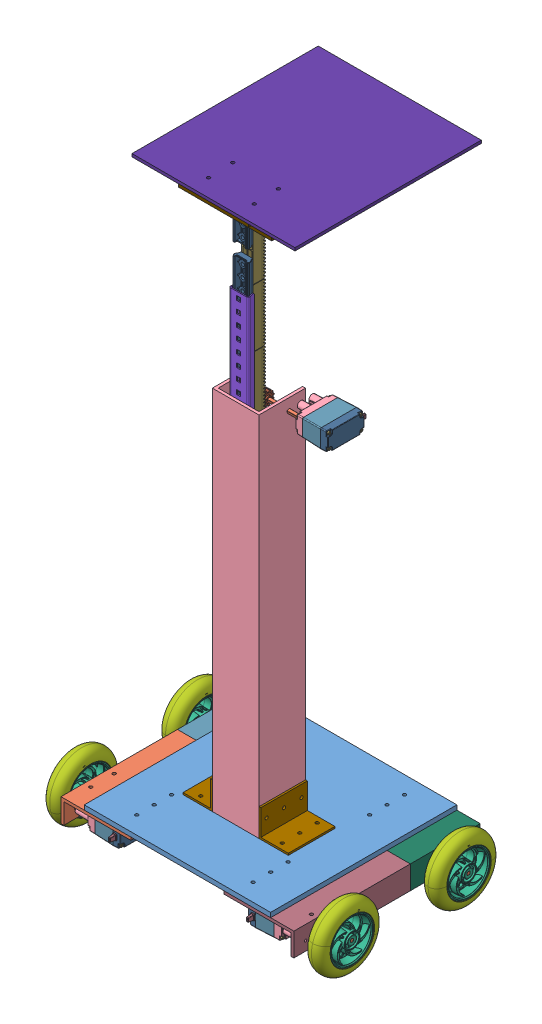
SolidWorks assembly mte380_Assy_01_lift_02., configuration Default. Lengths in mm.
Overall size (307.05 665.15 247.45).
138 component instances, 38 part files, 94 mates.
Components (placement in the parent):
- mte380_01_lift_base_02-1: mte380_01_lift_base_02 [Default] at (94.2351 110.2702 143.398) size (203.2 5 203.2)
- mte380_01_motor_bot_L_bracket_01-1: mte380_01_motor_bot_L_bracket_01 [Default] at (43.4351 110.2702 168.798) size (76.2 25.4 127)
- mte380_Assy_motor_vex_393_01-1: mte380_Assy_motor_vex_393_01 [Default] at (16.7501 95.0302 218.0279) x (0 0 -1) z (1 0 0) size (277.81 20.59 51.81)
  - SPPM206-0150BO-1: SPPM206-0150BO [Default] at (17.3 7.3 -1.5) x (1 0 0) z (0 -1 0) size (3.3 16.36 3.3)
  - 276-2181-003 Rev1-1: 276-2181-003 Rev1 [Default] at (0 0 -28) size (38.95 18.95 25.5)
  - 276-2177-019 Rev1-1: 276-2177-019 Rev1 [Default] at (-14.2702 0 -28) x (0.144195 -0.989549 0) z (0.989549 0.144195 0) size (6.3 15.8 6.3)
  - 276-2181-011 Rev1-1: 276-2181-011 Rev1 [Default] at (11.1298 0 -11) x (-1 0 0) z (0 1 0) size (11 4 11)
  - 276-2177-017 Rev1-1: 276-2177-017 Rev1 [Default] at (-245.51 0.1 2.5) size (248.21 15.59 2.54) (hidden)
  - QFK-N30QAV-16068-1: QFK-N30QAV-16068 [Default] at (-12.9 0 -23) x (0 1 0) z (0 0 1) size (12 10 26.1)
  - SPPM143-0030BO-1: SPPM143-0030BO [Default] at (-12.9 4.25 -6) x (-1 0 0) z (0 1 0) size (2.4 6.08 2.4)
  - 276-2181-010 Rev1-1: 276-2181-010 Rev1 [Default] at (10.8763 0 -9.4) x (0.878827 0.47714 0) z (0 0 1) size (1.5 1.5 16)
  - 276-2181-001 Rev1-1: 276-2181-001 Rev1 [Default] at origin size (40 20 8.01)
  - 276-2181-006 Rev1-1: 276-2181-006 Rev1 [Default] at (10.8763 0 -1.05) x (-0.259931 -0.965627 0) z (0 0 1) size (14.22 14.25 6.9)
  - 276-2181-007 Rev1-1: 276-2181-007 Rev1 [Default] at (2.1533 -1.4937 -4.4) x (-0.202497 0.979283 0) z (0 0 1) size (14.22 14.25 14.9)
  - 276-2181-010 Rev1-2: 276-2181-010 Rev1 [Default] at (-5.7003 2.586 -9.4) size (1.5 1.5 16)
  - 276-2177-018 Rev1-1: 276-2177-018 Rev1 [Default] at (-18.5 0.1 2.5) x (0 1 0) z (1 0 0) size (6.82 4.47 8.9)
  - 276-2181-006 Rev1-2: 276-2181-006 Rev1 [Default] at (2.1533 -1.4937 2.75) x (-0.071378 0.997449 0) z (0 0 1) size (14.22 14.25 6.9)
  - 276-2181-002 Rev1-1: 276-2181-002 Rev1 [Default] at (0 0 -20) size (40 20 23)
  - 276-2181-009 Rev1-1: 276-2181-009 Rev1 [Default] at (2.1533 -1.4937 -26.5) size (1.5 1.5 33)
  - SPPM206-0150BO-2: SPPM206-0150BO [Default] at (-16.9263 6.9263 -18.5) x (-0.075705 0.99713 0) z (-0.99713 -0.075705 0) size (3.3 16.36 3.3)
  - 276-2181-011 Rev1-2: 276-2181-011 Rev1 [Default] at (11.1298 0 -24) x (-0.997622 -0.068917 0) z (-0.068917 0.997622 0) size (11 4 11)
  - 276-2177-019 Rev1-2: 276-2177-019 Rev1 [Default] at (-1.5702 0 -28) x (0.32391 -0.946088 0) z (0.946088 0.32391 0) size (6.3 15.8 6.3)
  - SPPM206-0150BO-3: SPPM206-0150BO [Default] at (-17.3 -7.3 -1.5) x (0.292947 -0.956129 0) z (-0.956129 -0.292947 0) size (3.3 16.36 3.3)
  - SPPM206-0150BO-4: SPPM206-0150BO [Default] at (16.9263 -6.9263 -18.5) x (0.149257 -0.988799 0) z (0.988799 0.149257 0) size (3.3 16.36 3.3)
  - SPPM206-0150BO-5: SPPM206-0150BO [Default] at (17.3 -7.3 -1.5) x (1 0 0) z (0 -1 0) size (3.3 16.36 3.3)
  - SPPM206-0150BO-6: SPPM206-0150BO [Default] at (-16.9263 -6.9263 -18.5) x (-0.049887 0.998755 0) z (-0.998755 -0.049887 0) size (3.3 16.36 3.3)
  - SPPM206-0150BO-7: SPPM206-0150BO [Default] at (-17.3 7.3 -1.5) x (-0.963198 0.268794 0) z (0.268794 0.963198 0) size (3.3 16.36 3.3)
  - SPPM206-0150BO-8: SPPM206-0150BO [Default] at (16.9263 6.9263 -18.5) x (0.906825 0.421508 0) z (-0.421508 0.906825 0) size (3.3 16.36 3.3)
  - SPPM143-0030BO-2: SPPM143-0030BO [Default] at (-12.9 -4.25 -6) x (-0.988208 -0.153116 0) z (-0.153116 0.988208 0) size (2.4 6.08 2.4)
  - 276-2181-004 Rev1-1: 276-2181-004 Rev1 [Default] at (-12.9 0 -0.1) x (0.94341 -0.331628 0) z (0 0 -1) size (5.17 5.4 3)
  - 276-2181-005 Rev1-1: 276-2181-005 Rev1 [Default] at (-5.7003 2.586 -0.05) x (0.460478 -0.887671 0) z (0 0 1) size (11.88 11.88 5.9)
  - 276-2181-008 Rev1_276-2181-008g-1: 276-2181-008 Rev1_276-2181-008g [Default] at (11.1298 0 -14.5) x (0.267616 -0.963526 0) z (0 0 -1) size (13.83 13.88 17.3)
  - 276-2181-012 Rev1-1: 276-2181-012 Rev1 [Default] at (-12.9 0 -24) size (13.6 13 1)
- mte380_01_vex_shaft_2-1: mte380_01_vex_shaft_2 [Default] at (-31.9499 95.0479 206.9293) x (0 -0.267616 0.963526) z (-1 0 0) size (4.18 4.18 51.01)
- mte380_01_vex_bearing_block-1: mte380_01_vex_bearing_block [Default] at (-24.8662 107.0952 130.6495) x (0 0 -1) z (0 -1 0) size (35.56 10.16 13.39)
- mte380_01_center_shaft_01-1: mte380_01_center_shaft_01 [Default] at (68.8351 115.2702 130.698) size (50.8 400 50.8)
- mte380_Assy_wheel_vex_275-1: mte380_Assy_wheel_vex_275 [Default] at (-45.4869 83.9602 188.1506) x (0 0.267616 -0.963526) z (1 0 0) size (69.86 69.86 20.66)
  - SMALL-WHEEL-RIM-1: SMALL-WHEEL-RIM [Default] at (-15.1515 15.6838 -2.6601) size (61.43 61.43 9.24)
  - SMALL-WHEEL-HUB-1: SMALL-WHEEL-HUB [Default] at (-15.1515 15.6838 -2.6601) size (61.36 61.43 20.66)
  - SMALL-WHEEL-TIRE-1: SMALL-WHEEL-TIRE [Default] at (-15.1515 15.6838 -2.6601) x (1 0 0) z (0 -1 0) size (69.86 19.99 69.86)
- mte380_01_vex_rack_guide-1: mte380_01_vex_rack_guide [Default] at (94.2351 324.7702 178.323) x (-1 0 0) z (0 0 -1) size (20.84 444.5 8.8)
- mte380_01_vert_rack_bracket_01-1: mte380_01_vert_rack_bracket_01 [Default] at (119.6351 145.2702 130.698) size (32 30 50.8)
- mte380_01_vert_rack_bracket_01-2: mte380_01_vert_rack_bracket_01 [Default] at (68.8351 145.2702 181.498) x (-1 0 0) z (0 0 -1) size (32 30 50.8)
- mte380_01_vex_rack_slide-1: mte380_01_vex_rack_slide [Default] at (94.2351 622.1608 173.3216) x (1 0 0) z (0 1 0) size (17.45 8.37 50.79)
- mte380_01_vex_pinion_12-1: mte380_01_vex_pinion_12 [Default] at (93.6302 502.9979 149.2208) x (0 0.267616 -0.963526) z (1 0 0) size (14.8 14.8 9.53)
- mte380_01_vex_rack-1: mte380_01_vex_rack [Default] at (94.2351 653.9108 168.7501) x (0 1 0) z (-1 0 0) size (63 14.6 12.7)
- mte380_01_vex_rack_slide-2: mte380_01_vex_rack_slide [Default] at (94.2351 685.6608 173.3216) x (1 0 0) z (0 1 0) size (17.45 8.37 50.79)
- mte380_01_motor_bot_R_bracket_01-1: mte380_01_motor_bot_R_bracket_01 [Default] at (145.0351 110.2702 244.998) x (-1 0 0) z (0 0 -1) size (76.2 25.4 127)
- mte380_Assy_motor_vex_393_01-2: mte380_Assy_motor_vex_393_01 [Default] at (172.3201 95.0302 218.0279) x (0 0 -1) z (-1 0 0) size (277.81 20.59 51.81)
  - SPPM206-0150BO-1: SPPM206-0150BO [Default] at (17.3 7.3 -1.5) x (1 0 0) z (0 -1 0) size (3.3 16.36 3.3)
  - 276-2181-003 Rev1-1: 276-2181-003 Rev1 [Default] at (0 0 -28) size (38.95 18.95 25.5)
  - 276-2177-019 Rev1-1: 276-2177-019 Rev1 [Default] at (-14.2702 0 -28) x (0.144195 -0.989549 0) z (0.989549 0.144195 0) size (6.3 15.8 6.3)
  - 276-2181-011 Rev1-1: 276-2181-011 Rev1 [Default] at (11.1298 0 -11) x (-1 0 0) z (0 1 0) size (11 4 11)
  - 276-2177-017 Rev1-1: 276-2177-017 Rev1 [Default] at (-245.51 0.1 2.5) size (248.21 15.59 2.54) (hidden)
  - QFK-N30QAV-16068-1: QFK-N30QAV-16068 [Default] at (-12.9 0 -23) x (0 1 0) z (0 0 1) size (12 10 26.1)
  - SPPM143-0030BO-1: SPPM143-0030BO [Default] at (-12.9 4.25 -6) x (-1 0 0) z (0 1 0) size (2.4 6.08 2.4)
  - 276-2181-010 Rev1-1: 276-2181-010 Rev1 [Default] at (10.8763 0 -9.4) x (0.878827 0.47714 0) z (0 0 1) size (1.5 1.5 16)
  - 276-2181-001 Rev1-1: 276-2181-001 Rev1 [Default] at origin size (40 20 8.01)
  - 276-2181-006 Rev1-1: 276-2181-006 Rev1 [Default] at (10.8763 0 -1.05) x (-0.259931 -0.965627 0) z (0 0 1) size (14.22 14.25 6.9)
  - 276-2181-007 Rev1-1: 276-2181-007 Rev1 [Default] at (2.1533 -1.4937 -4.4) x (-0.202497 0.979283 0) z (0 0 1) size (14.22 14.25 14.9)
  - 276-2181-010 Rev1-2: 276-2181-010 Rev1 [Default] at (-5.7003 2.586 -9.4) size (1.5 1.5 16)
  - 276-2177-018 Rev1-1: 276-2177-018 Rev1 [Default] at (-18.5 0.1 2.5) x (0 1 0) z (1 0 0) size (6.82 4.47 8.9)
  - 276-2181-006 Rev1-2: 276-2181-006 Rev1 [Default] at (2.1533 -1.4937 2.75) x (-0.071378 0.997449 0) z (0 0 1) size (14.22 14.25 6.9)
  - 276-2181-002 Rev1-1: 276-2181-002 Rev1 [Default] at (0 0 -20) size (40 20 23)
  - 276-2181-009 Rev1-1: 276-2181-009 Rev1 [Default] at (2.1533 -1.4937 -26.5) size (1.5 1.5 33)
  - SPPM206-0150BO-2: SPPM206-0150BO [Default] at (-16.9263 6.9263 -18.5) x (-0.075705 0.99713 0) z (-0.99713 -0.075705 0) size (3.3 16.36 3.3)
  - 276-2181-011 Rev1-2: 276-2181-011 Rev1 [Default] at (11.1298 0 -24) x (-0.997622 -0.068917 0) z (-0.068917 0.997622 0) size (11 4 11)
  - 276-2177-019 Rev1-2: 276-2177-019 Rev1 [Default] at (-1.5702 0 -28) x (0.32391 -0.946088 0) z (0.946088 0.32391 0) size (6.3 15.8 6.3)
  - SPPM206-0150BO-3: SPPM206-0150BO [Default] at (-17.3 -7.3 -1.5) x (0.292947 -0.956129 0) z (-0.956129 -0.292947 0) size (3.3 16.36 3.3)
  - SPPM206-0150BO-4: SPPM206-0150BO [Default] at (16.9263 -6.9263 -18.5) x (0.149257 -0.988799 0) z (0.988799 0.149257 0) size (3.3 16.36 3.3)
  - SPPM206-0150BO-5: SPPM206-0150BO [Default] at (17.3 -7.3 -1.5) x (1 0 0) z (0 -1 0) size (3.3 16.36 3.3)
  - SPPM206-0150BO-6: SPPM206-0150BO [Default] at (-16.9263 -6.9263 -18.5) x (-0.049887 0.998755 0) z (-0.998755 -0.049887 0) size (3.3 16.36 3.3)
  - SPPM206-0150BO-7: SPPM206-0150BO [Default] at (-17.3 7.3 -1.5) x (-0.963198 0.268794 0) z (0.268794 0.963198 0) size (3.3 16.36 3.3)
  - SPPM206-0150BO-8: SPPM206-0150BO [Default] at (16.9263 6.9263 -18.5) x (0.906825 0.421508 0) z (-0.421508 0.906825 0) size (3.3 16.36 3.3)
  - SPPM143-0030BO-2: SPPM143-0030BO [Default] at (-12.9 -4.25 -6) x (-0.988208 -0.153116 0) z (-0.153116 0.988208 0) size (2.4 6.08 2.4)
  - 276-2181-004 Rev1-1: 276-2181-004 Rev1 [Default] at (-12.9 0 -0.1) x (0.94341 -0.331628 0) z (0 0 -1) size (5.17 5.4 3)
  - 276-2181-005 Rev1-1: 276-2181-005 Rev1 [Default] at (-5.7003 2.586 -0.05) x (0.460478 -0.887671 0) z (0 0 1) size (11.88 11.88 5.9)
  - 276-2181-008 Rev1_276-2181-008g-1: 276-2181-008 Rev1_276-2181-008g [Default] at (11.1298 0 -14.5) x (0.267616 -0.963526 0) z (0 0 -1) size (13.83 13.88 17.3)
  - 276-2181-012 Rev1-1: 276-2181-012 Rev1 [Default] at (-12.9 0 -24) size (13.6 13 1)
- mte380_01_vex_shaft_2-2: mte380_01_vex_shaft_2 [Default] at (221.0201 95.0615 206.9157) x (0 0.267616 0.963526) z (-1 0 0) size (4.18 4.18 51.01)
- mte380_Assy_wheel_vex_275-4: mte380_Assy_wheel_vex_275 [Default] at (239.8772 75.9124 196.4833) x (0 -0.267616 -0.963526) z (1 0 0) size (69.86 69.86 20.66)
  - SMALL-WHEEL-RIM-1: SMALL-WHEEL-RIM [Default] at (-15.1515 15.6838 -2.6601) size (61.43 61.43 9.24)
  - SMALL-WHEEL-HUB-1: SMALL-WHEEL-HUB [Default] at (-15.1515 15.6838 -2.6601) size (61.36 61.43 20.66)
  - SMALL-WHEEL-TIRE-1: SMALL-WHEEL-TIRE [Default] at (-15.1515 15.6838 -2.6601) x (1 0 0) z (0 -1 0) size (69.86 19.99 69.86)
- mte380_01_vex_shaft_2-3: mte380_01_vex_shaft_2 [Default] at (221.2351 95.0937 79.8345) x (0 0 1) z (-1 0 0) size (4.18 4.18 51.01)
- mte380_01_vex_shaft_2-4: mte380_01_vex_shaft_2 [Default] at (-32.7649 95.1912 79.8345) x (0 0 1) z (-1 0 0) size (4.18 4.18 51.01)
- mte380_01_front_bot_L_bracket_01-1: mte380_01_front_bot_L_bracket_01 [Default] at (43.4351 110.2702 41.798) size (76.2 25.4 76.2)
- mte380_01_front_bot_R_bracket_01-1: mte380_01_front_bot_R_bracket_01 [Default] at (145.0351 110.2702 117.998) x (-1 0 0) z (0 0 -1) size (76.2 25.4 76.2)
- mte380_01_vex_flat_bearing-2: mte380_01_vex_flat_bearing [Default] at (129.0839 107.7302 106.314) x (1 0 0) z (0 1 0) size (7.04 35.56 10.16)
- mte380_01_vex_flat_bearing-3: mte380_01_vex_flat_bearing [Default] at (59.3863 107.7302 53.482) x (-1 0 0) z (0 1 0) size (7.04 35.56 10.16)
- mte380_Assy_wheel_vex_275-5: mte380_Assy_wheel_vex_275 [Default] at (-46.3019 79.4824 64.708) x (0 0 -1) z (1 0 0) size (69.86 69.86 20.66)
  - SMALL-WHEEL-RIM-1: SMALL-WHEEL-RIM [Default] at (-15.1515 15.6838 -2.6601) size (61.43 61.43 9.24)
  - SMALL-WHEEL-HUB-1: SMALL-WHEEL-HUB [Default] at (-15.1515 15.6838 -2.6601) size (61.36 61.43 20.66)
  - SMALL-WHEEL-TIRE-1: SMALL-WHEEL-TIRE [Default] at (-15.1515 15.6838 -2.6601) x (1 0 0) z (0 -1 0) size (69.86 19.99 69.86)
- mte380_Assy_wheel_vex_275-6: mte380_Assy_wheel_vex_275 [Default] at (240.0922 79.4349 64.658) x (0 0 -1) z (1 0 0) size (69.86 69.86 20.66)
  - SMALL-WHEEL-RIM-1: SMALL-WHEEL-RIM [Default] at (-15.1515 15.6838 -2.6601) size (61.43 61.43 9.24)
  - SMALL-WHEEL-HUB-1: SMALL-WHEEL-HUB [Default] at (-15.1515 15.6838 -2.6601) size (61.36 61.43 20.66)
  - SMALL-WHEEL-TIRE-1: SMALL-WHEEL-TIRE [Default] at (-15.1515 15.6838 -2.6601) x (1 0 0) z (0 -1 0) size (69.86 19.99 69.86)
- mte380_Assy_motor_vex_393_01-3: mte380_Assy_motor_vex_393_01 [Default] at (163.3228 503.011 138.0423) x (0 0 1) z (1 0 0) size (277.81 20.59 51.81)
  - SPPM206-0150BO-1: SPPM206-0150BO [Default] at (17.3 7.3 -1.5) x (1 0 0) z (0 -1 0) size (3.3 16.36 3.3)
  - 276-2181-003 Rev1-1: 276-2181-003 Rev1 [Default] at (0 0 -28) size (38.95 18.95 25.5)
  - 276-2177-019 Rev1-1: 276-2177-019 Rev1 [Default] at (-14.2702 0 -28) x (0.144195 -0.989549 0) z (0.989549 0.144195 0) size (6.3 15.8 6.3)
  - 276-2181-011 Rev1-1: 276-2181-011 Rev1 [Default] at (11.1298 0 -11) x (-1 0 0) z (0 1 0) size (11 4 11)
  - 276-2177-017 Rev1-1: 276-2177-017 Rev1 [Default] at (-245.51 0.1 2.5) size (248.21 15.59 2.54) (hidden)
  - QFK-N30QAV-16068-1: QFK-N30QAV-16068 [Default] at (-12.9 0 -23) x (0 1 0) z (0 0 1) size (12 10 26.1)
  - SPPM143-0030BO-1: SPPM143-0030BO [Default] at (-12.9 4.25 -6) x (-1 0 0) z (0 1 0) size (2.4 6.08 2.4)
  - 276-2181-010 Rev1-1: 276-2181-010 Rev1 [Default] at (10.8763 0 -9.4) x (0.878827 0.47714 0) z (0 0 1) size (1.5 1.5 16)
  - 276-2181-001 Rev1-1: 276-2181-001 Rev1 [Default] at origin size (40 20 8.01)
  - 276-2181-006 Rev1-1: 276-2181-006 Rev1 [Default] at (10.8763 0 -1.05) x (-0.259931 -0.965627 0) z (0 0 1) size (14.22 14.25 6.9)
  - 276-2181-007 Rev1-1: 276-2181-007 Rev1 [Default] at (2.1533 -1.4937 -4.4) x (-0.202497 0.979283 0) z (0 0 1) size (14.22 14.25 14.9)
  - 276-2181-010 Rev1-2: 276-2181-010 Rev1 [Default] at (-5.7003 2.586 -9.4) size (1.5 1.5 16)
  - 276-2177-018 Rev1-1: 276-2177-018 Rev1 [Default] at (-18.5 0.1 2.5) x (0 1 0) z (1 0 0) size (6.82 4.47 8.9)
  - 276-2181-006 Rev1-2: 276-2181-006 Rev1 [Default] at (2.1533 -1.4937 2.75) x (-0.071378 0.997449 0) z (0 0 1) size (14.22 14.25 6.9)
  - 276-2181-002 Rev1-1: 276-2181-002 Rev1 [Default] at (0 0 -20) size (40 20 23)
  - 276-2181-009 Rev1-1: 276-2181-009 Rev1 [Default] at (2.1533 -1.4937 -26.5) size (1.5 1.5 33)
  - SPPM206-0150BO-2: SPPM206-0150BO [Default] at (-16.9263 6.9263 -18.5) x (-0.075705 0.99713 0) z (-0.99713 -0.075705 0) size (3.3 16.36 3.3)
  - 276-2181-011 Rev1-2: 276-2181-011 Rev1 [Default] at (11.1298 0 -24) x (-0.997622 -0.068917 0) z (-0.068917 0.997622 0) size (11 4 11)
  - 276-2177-019 Rev1-2: 276-2177-019 Rev1 [Default] at (-1.5702 0 -28) x (0.32391 -0.946088 0) z (0.946088 0.32391 0) size (6.3 15.8 6.3)
  - SPPM206-0150BO-3: SPPM206-0150BO [Default] at (-17.3 -7.3 -1.5) x (0.292947 -0.956129 0) z (-0.956129 -0.292947 0) size (3.3 16.36 3.3)
  - SPPM206-0150BO-4: SPPM206-0150BO [Default] at (16.9263 -6.9263 -18.5) x (0.149257 -0.988799 0) z (0.988799 0.149257 0) size (3.3 16.36 3.3)
  - SPPM206-0150BO-5: SPPM206-0150BO [Default] at (17.3 -7.3 -1.5) x (1 0 0) z (0 -1 0) size (3.3 16.36 3.3)
  - SPPM206-0150BO-6: SPPM206-0150BO [Default] at (-16.9263 -6.9263 -18.5) x (-0.049887 0.998755 0) z (-0.998755 -0.049887 0) size (3.3 16.36 3.3)
  - SPPM206-0150BO-7: SPPM206-0150BO [Default] at (-17.3 7.3 -1.5) x (-0.963198 0.268794 0) z (0.268794 0.963198 0) size (3.3 16.36 3.3)
  - SPPM206-0150BO-8: SPPM206-0150BO [Default] at (16.9263 6.9263 -18.5) x (0.906825 0.421508 0) z (-0.421508 0.906825 0) size (3.3 16.36 3.3)
  - SPPM143-0030BO-2: SPPM143-0030BO [Default] at (-12.9 -4.25 -6) x (-0.988208 -0.153116 0) z (-0.153116 0.988208 0) size (2.4 6.08 2.4)
  - 276-2181-004 Rev1-1: 276-2181-004 Rev1 [Default] at (-12.9 0 -0.1) x (0.94341 -0.331628 0) z (0 0 -1) size (5.17 5.4 3)
  - 276-2181-005 Rev1-1: 276-2181-005 Rev1 [Default] at (-5.7003 2.586 -0.05) x (0.460478 -0.887671 0) z (0 0 1) size (11.88 11.88 5.9)
  - 276-2181-008 Rev1_276-2181-008g-1: 276-2181-008 Rev1_276-2181-008g [Default] at (11.1298 0 -14.5) x (0.267616 -0.963526 0) z (0 0 -1) size (13.83 13.88 17.3)
  - 276-2181-012 Rev1-1: 276-2181-012 Rev1 [Default] at (-12.9 0 -24) size (13.6 13 1)
- mte380_01_vex_shaft_2-5: mte380_01_vex_shaft_2 [Default] at (114.6228 503.0287 149.2034) x (0 -0.267616 0.963526) z (-1 0 0) size (4.18 4.18 51.01)
- mte380_01_lift_platform_02-1: mte380_01_lift_platform_02 [Default] at (183.1351 713.9858 2.498) size (177.8 3.17 203.2)
- mte380_01_lift_platform__bracket_01-1: mte380_01_lift_platform__bracket_01 [Default] at (132.3351 685.4108 168.7501) x (0 0 1) z (-1 0 0) size (28.57 28.57 76.2)
- mte380_01_lift_platform__bracket_01-2: mte380_01_lift_platform__bracket_01 [Default] at (56.1351 685.4108 177.123) x (0 0 -1) z (1 0 0) size (28.57 28.57 76.2)
- mte380_01_vex_rack_slide-3: mte380_01_vex_rack_slide [Default] at (94.2351 495.1608 173.3216) x (1 0 0) z (0 1 0) size (17.45 8.37 50.79)
- mte380_01_vex_rack-2: mte380_01_vex_rack [Default] at (94.2351 526.9108 168.7501) x (0 1 0) z (-1 0 0) size (63 14.6 12.7)
- mte380_01_vex_rack_slide-4: mte380_01_vex_rack_slide [Default] at (94.2351 558.6608 173.3216) x (1 0 0) z (0 1 0) size (17.45 8.37 50.79)
- mte380_01_vex_rack-3: mte380_01_vex_rack [Default] at (94.2351 590.4108 168.7501) x (0 1 0) z (-1 0 0) size (63 14.6 12.7)
- Part2^mte380_Assy_01_lift_02.-1: Part2^mte380_Assy_01_lift_02. [Default] at (43.4351 110.2702 41.798) x (1 0 0) z (0 1 0) (virtual)
Mates (geometry in assembly coordinates):
- Coincident2: coincident: line of mte380_01_lift_base_02-1 through (-7.3649 110.2702 244.998) axis (1 0 0); plane of mte380_01_motor_bot_L_bracket_01-1 through (43.4351 110.2702 244.998) normal (0 0 1)
- Coincident7: coincident anti-aligned: plane of mte380_Assy_motor_vex_393_01-1/276-2181-008 Rev1_276-2181-008g-1 through (-6.5499 96.1526 208.8837) normal (0 0.267616 -0.963526); plane of mte380_01_vex_shaft_2-1 through (-57.3499 93.0935 208.034) normal (0 -0.267616 0.963526)
- Coincident8: coincident anti-aligned: plane of mte380_Assy_motor_vex_393_01-1/276-2181-008 Rev1_276-2181-008g-1 through (-6.5499 97.0159 205.7756) normal (0 -0.963526 -0.267616); plane of mte380_01_vex_shaft_2-1 through (-57.3499 97.0023 205.8245) normal (0 0.963526 0.267616)
- Coincident9: coincident anti-aligned: plane of mte380_Assy_motor_vex_393_01-1/276-2181-008 Rev1_276-2181-008g-1 through (-6.5499 93.0445 208.0204) normal (-1 0 0); plane of mte380_01_vex_shaft_2-1 through (-6.5499 97.0023 205.8245) normal (1 0 0)
- Coincident10: coincident anti-aligned: plane of mte380_01_lift_base_02-1 through (94.2351 110.2702 143.398) normal (0 -1 0); plane of mte380_01_motor_bot_L_bracket_01-1 through (43.4351 110.2702 244.998) normal (0 1 0)
- Coincident29: coincident aligned: plane of mte380_01_lift_base_02-1 through (-7.3649 115.2702 244.998) normal (0 0 1); plane of mte380_01_motor_bot_L_bracket_01-1 through (43.4351 110.2702 244.998) normal (0 0 1)
- Distance3: distance = 50.8 mm anti-aligned: plane of mte380_01_lift_base_02-1 through (-7.3649 115.2702 244.998) normal (-1 0 0); plane of mte380_01_motor_bot_L_bracket_01-1 through (43.4351 107.0952 244.998) normal (1 0 0)
- Distance5: distance = 2.54 mm anti-aligned: plane of mte380_Assy_motor_vex_393_01-1/276-2177-019 Rev1-2 through (-27.0499 95.0302 219.598) normal (-1 0 0); plane of mte380_01_motor_bot_L_bracket_01-1 through (-29.5899 84.8702 244.998) normal (1 0 0)
- Coincident48: coincident anti-aligned: plane of mte380_01_lift_base_02-1 through (94.2351 115.2702 143.398) normal (0 1 0); plane of mte380_01_center_shaft_01-1 through (68.8351 115.2702 130.698) normal (0 -1 0)
- Width1: width anti-aligned: plane of mte380_01_lift_base_02-1 through (-7.3649 115.2702 244.998) normal (-1 0 0); plane of mte380_01_lift_base_02-1 through (195.8351 115.2702 244.998) normal (1 0 0); plane of mte380_01_center_shaft_01-1 through (119.6351 515.2702 181.498) normal (1 0 0); plane of mte380_01_center_shaft_01-1 through (68.8351 515.2702 130.698) normal (-1 0 0)
- Distance6: distance = 63.5 mm aligned: plane of mte380_01_center_shaft_01-1 through (68.8351 515.2702 181.498) normal (0 0 1); plane of mte380_01_lift_base_02-1 through (-7.3649 115.2702 244.998) normal (0 0 1)
- Coincident52: coincident anti-aligned: plane of mte380_01_vex_shaft_2-1 through (-57.3499 93.9431 204.9748) normal (0 0.267616 -0.963526); plane of mte380_Assy_wheel_vex_275-1/SMALL-WHEEL-HUB-1 through (-36.717 93.895 204.9615) normal (0 -0.267616 0.963526)
- Coincident53: coincident anti-aligned: plane of mte380_01_vex_shaft_2-1 through (-57.3499 97.0023 205.8245) normal (0 0.963526 0.267616); plane of mte380_Assy_wheel_vex_275-1/SMALL-WHEEL-HUB-1 through (-36.717 97.0023 205.8245) normal (0 -0.963526 -0.267616)
- Tangent9: tangent anti-aligned: plane of mte380_01_vex_shaft_2-1 through (-57.3499 97.0023 205.8245) normal (-1 0 0); sphere of mte380_Assy_wheel_vex_275-1/SMALL-WHEEL-HUB-1
- Coincident55: coincident anti-aligned: plane of mte380_01_center_shaft_01-1 through (116.4601 515.2702 178.323) normal (0 0 -1); plane of mte380_01_vex_rack_guide-1 through (85.7693 172.3702 178.323) normal (0 0 1)
- Width2: width anti-aligned: plane of mte380_01_center_shaft_01-1 through (116.4601 515.2702 130.698) normal (-1 0 0); plane of mte380_01_center_shaft_01-1 through (72.0101 515.2702 178.323) normal (1 0 0); plane of mte380_01_vex_rack_guide-1 through (104.59 172.3702 175.861) normal (0.965926 0 -0.258819); plane of mte380_01_vex_rack_guide-1 through (85.5782 172.3702 169.5238) normal (-0.965926 0 -0.258819)
- Coincident56: coincident anti-aligned: plane of mte380_01_center_shaft_01-1 through (119.6351 515.2702 181.498) normal (1 0 0); plane of mte380_01_vert_rack_bracket_01-1 through (119.6351 145.2702 181.498) normal (-1 0 0)
- Coincident57: coincident anti-aligned: plane of mte380_01_lift_base_02-1 through (94.2351 115.2702 143.398) normal (0 1 0); plane of mte380_01_vert_rack_bracket_01-1 through (119.6351 115.2702 181.498) normal (0 -1 0)
- Coincident58: coincident anti-aligned: plane of mte380_01_center_shaft_01-1 through (68.8351 515.2702 130.698) normal (-1 0 0); plane of mte380_01_vert_rack_bracket_01-2 through (68.8351 145.2702 130.698) normal (1 0 0)
- Coincident59: coincident anti-aligned: plane of mte380_01_lift_base_02-1 through (94.2351 115.2702 143.398) normal (0 1 0); plane of mte380_01_vert_rack_bracket_01-2 through (68.8351 115.2702 130.698) normal (0 -1 0)
- Coincident61: coincident anti-aligned: plane of mte380_01_vex_rack_guide-1 through (102.7008 172.3702 177.123) normal (0 0 -1); plane of mte380_01_vex_rack_slide-1 through (94.2351 622.1608 177.123) normal (0 0 1)
- Width3: width anti-aligned: plane of mte380_01_vex_rack_slide-1 through (103.5283 647.5608 177.2489) normal (0.965926 0 -0.258819); plane of mte380_01_vex_rack_slide-1 through (87.0326 647.5608 169.446) normal (-0.965926 0 -0.258819); plane of mte380_01_vex_rack_guide-1 through (101.7328 172.3702 169.8344) normal (-0.965926 0 0.258819); plane of mte380_01_vex_rack_guide-1 through (85.0393 172.3702 176.1716) normal (0.965926 0 0.258819)
- Coincident63: coincident anti-aligned: plane of mte380_01_vex_rack_slide-1 through (101.5342 647.5608 168.7501) normal (0 0 -1); plane of mte380_01_vex_rack-1 through (94.2351 653.9108 168.7501) normal (0 0 1)
- Coincident64: coincident anti-aligned: plane of mte380_01_vex_rack_guide-1 through (102.7008 172.3702 177.123) normal (0 0 -1); plane of mte380_01_vex_rack_slide-2 through (94.2351 685.6608 177.123) normal (0 0 1)
- Width4: width anti-aligned: plane of mte380_01_vex_rack_slide-2 through (103.5283 711.0608 177.2489) normal (0.965926 0 -0.258819); plane of mte380_01_vex_rack_slide-2 through (87.0326 711.0608 169.446) normal (-0.965926 0 -0.258819); plane of mte380_01_vex_rack_guide-1 through (101.7328 172.3702 169.8344) normal (-0.965926 0 0.258819); plane of mte380_01_vex_rack_guide-1 through (85.0393 172.3702 176.1716) normal (0.965926 0 0.258819)
- Concentric9: concentric anti-aligned: cylinder of mte380_01_vex_rack_slide-1 through (94.2351 628.5108 168.7501) axis (0 0 -1) radius 1.85; cylinder of mte380_01_vex_rack-1 through (94.2351 628.5108 168.7501) axis (0 0 1) radius 2.25
- Concentric12: concentric anti-aligned: cylinder of mte380_01_vex_rack-1 through (94.2351 679.3108 168.7501) axis (0 0 1) radius 2.25; cylinder of mte380_01_vex_rack_slide-2 through (94.2351 679.3108 168.7501) axis (0 0 -1) radius 1.85
- Coincident65: coincident aligned: plane of mte380_01_center_shaft_01-1 through (119.6351 515.2702 130.698) normal (0 0 -1); plane of mte380_01_vert_rack_bracket_01-1 through (119.6351 145.2702 130.698) normal (0 0 -1)
- Coincident66: coincident aligned: plane of mte380_01_center_shaft_01-1 through (72.0101 515.2702 130.698) normal (0 0 -1); plane of mte380_01_vert_rack_bracket_01-2 through (68.8351 145.2702 130.698) normal (0 0 -1)
- Coincident67: coincident anti-aligned: plane of mte380_01_lift_base_02-1 through (94.2351 110.2702 143.398) normal (0 -1 0); plane of mte380_01_motor_bot_R_bracket_01-1 through (145.0351 110.2702 168.798) normal (0 1 0)
- Coincident68: coincident aligned: plane of mte380_01_lift_base_02-1 through (-7.3649 115.2702 244.998) normal (0 0 1); plane of mte380_01_motor_bot_R_bracket_01-1 through (145.0351 110.2702 244.998) normal (0 0 1)
- Distance7: distance = 50.8 mm: line of mte380_01_lift_base_02-1 through (195.8351 115.2702 244.998) axis (0 -1 0); line of mte380_01_motor_bot_R_bracket_01-1 through (145.0351 107.0952 244.998) axis (0 1 0)
- Concentric13: concentric aligned: cylinder of mte380_01_motor_bot_R_bracket_01-1 through (221.2351 95.0302 219.598) axis (1 0 0) radius 1.3526; cylinder of mte380_Assy_motor_vex_393_01-2/276-2177-019 Rev1-2 through (216.1201 95.0302 219.598) axis (1 0 0) radius 1.3526
- Concentric14: concentric aligned: cylinder of mte380_01_motor_bot_R_bracket_01-1 through (221.2351 95.0302 232.298) axis (1 0 0) radius 1.3526; cylinder of mte380_Assy_motor_vex_393_01-2/276-2177-019 Rev1-1 through (216.1201 95.0302 232.298) axis (1 0 0) radius 1.3526
- Distance8: distance = 2.54 mm anti-aligned: plane of mte380_Assy_motor_vex_393_01-2/276-2181-003 Rev1-1 through (215.5201 95.0302 218.0279) normal (1 0 0); plane of mte380_01_motor_bot_R_bracket_01-1 through (218.0601 84.8702 168.798) normal (-1 0 0)
- Coincident71: coincident anti-aligned: plane of mte380_Assy_motor_vex_393_01-2/276-2181-008 Rev1_276-2181-008g-1 through (195.6201 97.0159 208.0204) normal (1 0 0); plane of mte380_01_vex_shaft_2-2 through (195.6201 96.1662 204.9613) normal (-1 0 0)
- Coincident72: coincident anti-aligned: plane of mte380_Assy_motor_vex_393_01-2/276-2181-008 Rev1_276-2181-008g-1 through (195.6201 96.1526 204.9123) normal (0 -0.963526 0.267616); plane of mte380_01_vex_shaft_2-2 through (195.6201 96.1662 204.9613) normal (0 0.963526 -0.267616)
- Coincident73: coincident anti-aligned: plane of mte380_Assy_motor_vex_393_01-2/276-2181-008 Rev1_276-2181-008g-1 through (195.6201 93.9078 208.8837) normal (0 -0.267616 -0.963526); plane of mte380_01_vex_shaft_2-2 through (195.6201 93.9567 208.8701) normal (0 0.267616 0.963526)
- Coincident74: coincident anti-aligned: plane of mte380_01_vex_shaft_2-2 through (195.6201 93.107 205.8109) normal (0 -0.963526 0.267616); plane of mte380_Assy_wheel_vex_275-4/SMALL-WHEEL-HUB-1 through (248.6472 93.9567 208.8701) normal (0 0.963526 -0.267616)
- Coincident76: coincident anti-aligned: plane of mte380_01_vex_shaft_2-2 through (195.6201 93.9567 208.8701) normal (0 0.267616 0.963526); plane of ? through (248.6472 97.0641 208.0071) normal (0 -0.267616 -0.963526)
- Tangent11: tangent anti-aligned: plane of mte380_01_vex_shaft_2-2 through (246.4201 96.1662 204.9613) normal (1 0 0); unknown of ?
- Concentric17: concentric anti-aligned: cylinder of mte380_01_motor_bot_L_bracket_01-1 through (-25.5934 110.2702 219.598) axis (0 1 0) radius 1.7272; cone of mte380_01_vex_bearing_block-1 through (-25.5934 107.0952 219.598) axis (0 -1 0)
- Distance13: distance = 0 mm anti-aligned: plane of mte380_01_vex_bearing_block-1 through (-31.6896 107.0952 228.2341) normal (0 1 0); plane of mte380_01_motor_bot_L_bracket_01-1 through (-29.5899 107.0952 244.998) normal (0 -1 0)
- Concentric18: concentric aligned: cylinder of mte380_01_motor_bot_L_bracket_01-1 through (-32.7649 95.0302 232.298) axis (-1 0 0) radius 1.3526; circle of mte380_Assy_motor_vex_393_01-1/276-2177-019 Rev1-1
- Concentric19: concentric aligned: circle of mte380_01_motor_bot_L_bracket_01-1; circle of mte380_Assy_motor_vex_393_01-1/276-2177-019 Rev1-2
- Coincident99: coincident anti-aligned: plane of mte380_01_lift_base_02-1 through (94.2351 110.2702 143.398) normal (0 -1 0); plane of mte380_01_front_bot_L_bracket_01-1 through (43.4351 110.2702 117.998) normal (0 1 0)
- Coincident100: coincident aligned: plane of mte380_01_lift_base_02-1 through (-7.3649 115.2702 41.798) normal (0 0 -1); plane of mte380_01_front_bot_L_bracket_01-1 through (43.4351 110.2702 41.798) normal (0 0 -1)
- Distance14: distance = 50.8 mm anti-aligned: plane of mte380_01_front_bot_L_bracket_01-1 through (43.4351 107.0952 117.998) normal (1 0 0); plane of mte380_01_lift_base_02-1 through (-7.3649 115.2702 244.998) normal (-1 0 0)
- Coincident102: coincident anti-aligned: plane of mte380_01_lift_base_02-1 through (94.2351 110.2702 143.398) normal (0 -1 0); plane of mte380_01_front_bot_R_bracket_01-1 through (145.0351 110.2702 41.798) normal (0 1 0)
- Coincident103: coincident aligned: plane of mte380_01_lift_base_02-1 through (-7.3649 115.2702 41.798) normal (0 0 -1); plane of mte380_01_front_bot_R_bracket_01-1 through (145.0351 110.2702 41.798) normal (0 0 -1)
- Distance16: distance = 50.8 mm anti-aligned: plane of mte380_01_front_bot_R_bracket_01-1 through (145.0351 107.0952 41.798) normal (-1 0 0); plane of mte380_01_lift_base_02-1 through (195.8351 115.2702 244.998) normal (1 0 0)
- Concentric20: concentric anti-aligned: cylinder of mte380_01_front_bot_R_bracket_01-1 through (221.2351 95.0302 67.198) axis (1 0 0) radius 1.7272; circle of mte380_01_vex_flat_bearing-2
- Coincident106: coincident anti-aligned: plane of mte380_01_front_bot_R_bracket_01-1 through (218.0601 84.8702 41.798) normal (-1 0 0); plane of mte380_01_vex_flat_bearing-2 through (218.0601 107.7302 106.314) normal (1 0 0)
- Concentric21: concentric anti-aligned: circle of mte380_01_front_bot_R_bracket_01-1; cylinder of mte380_01_vex_flat_bearing-2 through (211.7101 95.0302 92.598) axis (-1 0 0) radius 2.1209
- Concentric22: concentric anti-aligned: cylinder of mte380_01_front_bot_L_bracket_01-1 through (-32.7649 95.0302 67.198) axis (-1 0 0) radius 1.7272; cylinder of mte380_01_vex_flat_bearing-3 through (-23.2399 95.0302 67.198) axis (1 0 0) radius 2.1209
- Concentric23: concentric anti-aligned: cylinder of mte380_01_front_bot_L_bracket_01-1 through (-32.7649 95.0302 92.598) axis (-1 0 0) radius 1.7272; cylinder of mte380_01_vex_flat_bearing-3 through (-23.2399 95.0302 92.598) axis (1 0 0) radius 2.1209
- Coincident107: coincident anti-aligned: plane of mte380_01_front_bot_L_bracket_01-1 through (-29.5899 84.8702 117.998) normal (1 0 0); plane of mte380_01_vex_flat_bearing-3 through (-29.5899 107.7302 53.482) normal (-1 0 0)
- Coincident108: coincident anti-aligned: plane of mte380_01_vex_shaft_2-4 through (-58.1649 93.6037 78.247) normal (0 0 -1); plane of mte380_Assy_wheel_vex_275-5/SMALL-WHEEL-HUB-1 through (-37.532 93.5537 78.247) normal (0 0 1)
- Coincident109: coincident anti-aligned: plane of mte380_01_vex_shaft_2-4 through (-58.1649 96.7787 78.247) normal (0 1 0); plane of ? through (-37.532 96.7787 78.247) normal (0 -1 0)
- Tangent12: tangent anti-aligned: plane of mte380_01_vex_shaft_2-4 through (-58.1649 96.7787 78.247) normal (-1 0 0); sphere of ?
- Coincident110: coincident anti-aligned: plane of mte380_01_vex_shaft_2-3 through (195.8351 93.5062 81.422) normal (0 0 1); plane of mte380_Assy_wheel_vex_275-6/SMALL-WHEEL-HUB-1 through (248.8622 96.7312 81.422) normal (0 0 -1)
- Coincident111: coincident anti-aligned: plane of mte380_01_vex_shaft_2-3 through (195.8351 93.5062 78.247) normal (0 -1 0); plane of ? through (248.8622 93.5062 81.422) normal (0 1 0)
- Tangent13: tangent anti-aligned: plane of mte380_01_vex_shaft_2-3 through (246.6351 96.6812 78.247) normal (1 0 0); sphere of ?
- Coincident125: coincident anti-aligned: plane of mte380_Assy_motor_vex_393_01-3/276-2181-008 Rev1_276-2181-008g-1 through (140.0228 504.1334 151.1578) normal (0 -0.963526 -0.267616); plane of mte380_01_vex_shaft_2-5 through (89.2228 504.9831 148.0986) normal (0 0.963526 0.267616)
- Coincident126: coincident anti-aligned: plane of mte380_Assy_motor_vex_393_01-3/276-2181-008 Rev1_276-2181-008g-1 through (140.0228 501.0253 150.2945) normal (0 0.267616 -0.963526); plane of mte380_01_vex_shaft_2-5 through (89.2228 501.0742 150.3081) normal (0 -0.267616 0.963526)
- Coincident127: coincident anti-aligned: plane of mte380_Assy_motor_vex_393_01-3/276-2181-008 Rev1_276-2181-008g-1 through (140.0228 504.9967 148.0497) normal (-1 0 0); plane of mte380_01_vex_shaft_2-5 through (140.0228 504.9831 148.0986) normal (1 0 0)
- Coincident129: coincident anti-aligned: plane of mte380_01_vex_pinion_12-1 through (98.3927 504.3468 147.9219) normal (0 -0.267616 0.963526); plane of mte380_01_vex_shaft_2-5 through (89.2228 501.9239 147.2489) normal (0 0.267616 -0.963526)
- Coincident130: coincident anti-aligned: plane of mte380_01_vex_pinion_12-1 through (98.3927 504.2968 150.5697) normal (0 -0.963526 -0.267616); plane of mte380_01_vex_shaft_2-5 through (89.2228 504.9831 148.0986) normal (0 0.963526 0.267616)
- Distance17: distance = 101.6 mm aligned: plane of mte380_01_vex_rack_guide-1 through (85.7693 616.8702 176.3672) normal (0 1 0); plane of mte380_01_center_shaft_01-1 through (68.8351 515.2702 130.698) normal (0 1 0)
- Coincident135: coincident anti-aligned: plane of mte380_01_vex_rack_slide-2 through (101.5342 711.0608 168.7501) normal (0 0 -1); plane of mte380_01_lift_platform__bracket_01-1 through (56.1351 685.4108 168.7501) normal (0 0 1)
- Width6: width anti-aligned: plane of mte380_01_vex_rack_slide-2 through (87.5934 711.0608 169.4201) normal (-0.965926 0 -0.258819); plane of mte380_01_vex_rack_slide-2 through (100.8768 711.0608 169.4201) normal (0.965926 0 -0.258819); plane of mte380_01_lift_platform__bracket_01-1 through (132.3351 685.4108 168.7501) normal (1 0 0); plane of mte380_01_lift_platform__bracket_01-1 through (56.1351 685.4108 168.7501) normal (-1 0 0)
- Coincident136: coincident anti-aligned: plane of mte380_01_vex_rack-1 through (87.8851 685.4108 93.3328) normal (0 1 0); plane of mte380_01_lift_platform__bracket_01-1 through (56.1351 685.4108 165.5751) normal (0 -1 0)
- Coincident137: coincident anti-aligned: plane of mte380_01_vex_rack_slide-2 through (94.2351 685.6608 177.123) normal (0 0 1); plane of mte380_01_lift_platform__bracket_01-2 through (132.3351 685.4108 177.123) normal (0 0 -1)
- Coincident138: coincident aligned: plane of mte380_01_lift_platform__bracket_01-1 through (56.1351 713.9858 168.7501) normal (0 1 0); plane of mte380_01_lift_platform__bracket_01-2 through (132.3351 713.9858 177.123) normal (0 1 0)
- Width7: width anti-aligned: plane of mte380_01_vex_rack_slide-2 through (87.0326 711.0608 169.446) normal (-0.965926 0 -0.258819); plane of mte380_01_vex_rack_slide-2 through (103.5283 711.0608 177.2489) normal (0.965926 0 -0.258819); plane of mte380_01_lift_platform__bracket_01-2 through (132.3351 685.4108 177.123) normal (1 0 0); plane of mte380_01_lift_platform__bracket_01-2 through (56.1351 685.4108 177.123) normal (-1 0 0)
- Coincident139: coincident anti-aligned: plane of mte380_01_lift_platform_02-1 through (183.1351 713.9858 2.498) normal (0 -1 0); plane of mte380_01_lift_platform__bracket_01-1 through (56.1351 713.9858 168.7501) normal (0 1 0)
- Coincident140: coincident: line of mte380_01_vex_rack_guide-1 through (102.7008 616.8702 177.123) axis (-1 0 0); plane of mte380_01_lift_platform__bracket_01-2 through (132.3351 616.8702 183.473) normal (0 -1 0)
- Width8: width anti-aligned: plane of mte380_01_lift_platform__bracket_01-1 through (56.1351 685.4108 168.7501) normal (-1 0 0); plane of mte380_01_lift_platform__bracket_01-1 through (132.3351 685.4108 168.7501) normal (1 0 0); plane of mte380_01_lift_platform_02-1 through (183.1351 717.1608 2.498) normal (1 0 0); plane of mte380_01_lift_platform_02-1 through (5.3351 717.1608 2.498) normal (-1 0 0)
- Coincident142: coincident anti-aligned: plane of mte380_01_vex_rack_guide-1 through (102.7008 172.3702 177.123) normal (0 0 -1); plane of mte380_01_vex_rack_slide-3 through (94.2351 495.1608 177.123) normal (0 0 1)
- Concentric28: concentric anti-aligned: cylinder of mte380_01_vex_rack_slide-3 through (94.2351 501.5108 168.7501) axis (0 0 -1) radius 1.85; cylinder of mte380_01_vex_rack-2 through (94.2351 501.5108 168.7501) axis (0 0 1) radius 2.25
- Coincident143: coincident anti-aligned: plane of mte380_01_vex_rack_slide-3 through (101.5342 520.5608 168.7501) normal (0 0 -1); plane of mte380_01_vex_rack-2 through (94.2351 526.9108 168.7501) normal (0 0 1)
- Concentric31: concentric anti-aligned: cylinder of mte380_01_vex_rack-2 through (94.2351 552.3108 168.7501) axis (0 0 1) radius 2.25; cylinder of mte380_01_vex_rack_slide-4 through (94.2351 552.3108 168.7501) axis (0 0 -1) radius 1.85
- Coincident144: coincident anti-aligned: plane of mte380_01_vex_rack-2 through (94.2351 526.9108 168.7501) normal (0 0 1); plane of mte380_01_vex_rack_slide-4 through (101.5342 584.0608 168.7501) normal (0 0 -1)
- Coincident145: coincident anti-aligned: plane of mte380_01_vex_rack_guide-1 through (102.7008 172.3702 177.123) normal (0 0 -1); plane of mte380_01_vex_rack_slide-4 through (94.2351 558.6608 177.123) normal (0 0 1)
- Width9: width anti-aligned: plane of mte380_01_vex_rack_slide-4 through (103.5283 584.0608 177.2489) normal (0.965926 0 -0.258819); plane of mte380_01_vex_rack_slide-4 through (87.0326 584.0608 169.446) normal (-0.965926 0 -0.258819); plane of mte380_01_vex_rack_guide-1 through (101.7328 172.3702 169.8344) normal (-0.965926 0 0.258819); plane of mte380_01_vex_rack_guide-1 through (85.0393 172.3702 176.1716) normal (0.965926 0 0.258819)
- Concentric32: concentric anti-aligned: cylinder of mte380_01_vex_rack-2 through (94.2351 539.6108 169.7501) axis (0 0 1) radius 1.2573; cylinder of mte380_01_vex_rack_slide-4 through (94.2351 539.6108 168.7501) axis (0 0 -1) radius 2.1
- Concentric34: concentric anti-aligned: cylinder of mte380_01_vex_rack_slide-1 through (94.2351 615.8108 168.7501) axis (0 0 -1) radius 2.1; circle of mte380_01_vex_rack-3
- Concentric35: concentric anti-aligned: circle of mte380_01_vex_rack_slide-4; cylinder of mte380_01_vex_rack-3 through (94.2351 565.0108 168.7501) axis (0 0 1) radius 2.25
- Coincident147: coincident anti-aligned: plane of mte380_01_vex_rack_slide-1 through (101.5342 647.5608 168.7501) normal (0 0 -1); plane of mte380_01_vex_rack-3 through (94.2351 590.4108 168.7501) normal (0 0 1)
- InPlace1: in place: plane of mte380_01_front_bot_L_bracket_01-1 through (43.4351 110.2702 117.998) normal (0 1 0); plane of ? through (0 110.2702 0) normal (0 1 0); moOrthogonalPlaneRef_w of mte380_01_front_bot_L_bracket_01-1 through (43.4351 110.2702 117.998) normal (0 1 0); plane of ? through (0 110.2702 0) normal (0 0 -1); plane of mte380_01_front_bot_L_bracket_01-1 through (43.4351 110.2702 117.998) normal (0 1 0); line of ? through (-55 0 110.2702) axis (0 1 0); plane of mte380_01_front_bot_L_bracket_01-1 through (43.4351 110.2702 117.998) normal (0 1 0); unknown of Part2^mte380_Assy_01_lift_02.-1
- Coincident148: coincident aligned: plane of ?; plane of Part2^mte380_Assy_01_lift_02.-1
- Coincident149: coincident aligned: plane of mte380_01_front_bot_L_bracket_01-1 through (43.4351 110.2702 41.798) normal (0 0 -1); plane of Part2^mte380_Assy_01_lift_02.-1 through (43.4351 110.2702 41.798) normal (0 0 -1)
- Coincident150: coincident anti-aligned: plane of mte380_01_front_bot_L_bracket_01-1 through (43.4351 110.2702 41.798) normal (-1 0 0); unknown of Part2^mte380_Assy_01_lift_02.-1
- Concentric36: concentric anti-aligned: cylinder of mte380_01_lift_platform_02-1 through (69.8467 717.1608 186.648) axis (0 1 0) radius 1.7272; cylinder of mte380_01_lift_platform__bracket_01-2 through (69.8467 710.8108 186.648) axis (0 -1 0) radius 1.7272
